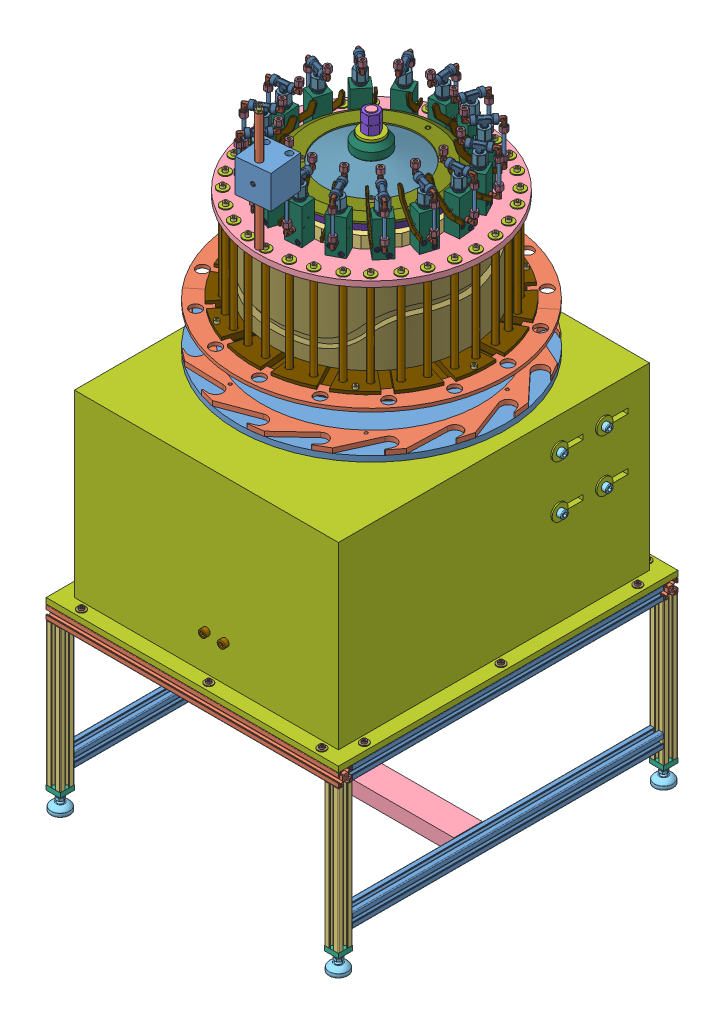
SolidWorks assembly Assieme_FINALE, configuration Default. Lengths in mm. (continued)
Components (placement in the parent): (continued)
- assieme parte rotante-2: assieme parte rotante [Default] at (-79.201 623.9178 -645.7922) x (0 1 0) z (-0.73003 0 0.683415) size (749.63 778.63 778.63) (continued)
  - AssiemeValvola-16: AssiemeValvola [Default] at (515.3257 153.2338 311.5106) x (0 -0.793353 0.608761) z (0 0.608761 0.793353) size (90.26 138.63 38) (continued)
    - Raccordo a L-2: Raccordo a L [Default] at (30 0 0) x (0 1 0) z (0 0 -1) size (28.34 25.51 14.01)
      - 1809_06_10_01-1: 1809_06_10_01 [Default] at origin size (22.49 23 10)
      - 1809_06_10_02-1: 1809_06_10_02 [Default] at origin size (6.5 8.5 8.5)
      - 1809_06_10_03-1: 1809_06_10_03 [Default] at origin size (11.02 15.01 14.01)
    - TappoChiusura-1: TappoChiusura [Default] at (0 -32 0) x (0 -1 0) z (0 0 1) size (38.28 26.74 26.74)
    - CorpoValvola-1: CorpoValvola [Default] at (-15 -115.2824 0) size (30 75 34)
    - Raccordo a L-3: Raccordo a L [Default] at (-30 -88.2824 0) x (0 1 0) z (0 0 1) size (28.34 25.51 14.01)
      - 1809_06_10_01-1: 1809_06_10_01 [Default] at origin size (22.49 23 10)
      - 1809_06_10_02-1: 1809_06_10_02 [Default] at origin size (6.5 8.5 8.5)
      - 1809_06_10_03-1: 1809_06_10_03 [Default] at origin size (11.02 15.01 14.01)
    - Spina_3x38-1: Spina_3x38 [Default] at (0 -68.2824 -21) x (-1 0 0) z (0 0 1) size (3 3 38)
    - Spina_3x38-2: Spina_3x38 [Default] at (-10 -80.2824 -21) x (0.996193 0.087174 0) z (0 0 1) size (3 3 38)
    - M5 40mm-3: M5 40mm [ISO 4762 M5 x 40 - 40N] at (-14.6 -108.7824 9) size (45 8.5 8.5)
    - M5 40mm-2: M5 40mm [ISO 4762 M5 x 40 - 40N] at (-14.6 -96.7824 -9) size (45 8.5 8.5)
    - LevaValvola-1: LevaValvola [Default] at (-24.507 -86.571 -17) x (0.996193 0.087174 0) z (0 0 1) size (77.55 60.2 4)
    - Tubo-1: Tubo [Default] at (-30 -15.9665 0) x (1 0 0) z (0 -1 0) size (6 6 56.4)
  - Disco alimentazione guarnizione fi24.4-1: Disco alimentazione guarnizione fi24.4 [Default] at (198.0433 18.3637 415) x (0 0.065403 0.997859) z (-1 0 0) size (570 285 7.35)
  - Disco alimentazione guarnizione fi24.4-2: Disco alimentazione guarnizione fi24.4 [Default] at (198.0433 18.3637 415) x (0 -0.065403 -0.997859) z (-1 0 0) size (570 285 7.35)
  - m6 12mm-1: m6 12mm [ISO 4762 M6 x 12 - 12N] at (210.0433 200.6849 574.8914) x (-1 0 0) z (0 0.793353 -0.608761) size (18 10 10)
  - m6 12mm-7: m6 12mm [ISO 4762 M6 x 12 - 12N] at (210.0433 260.3445 399.1397) x (-1 0 0) z (0 0.793353 -0.608761) size (18 10 10)
  - m6 12mm-8: m6 12mm [ISO 4762 M6 x 12 - 12N] at (210.0433 96.3128 185.3694) x (-1 0 0) z (0 0.793353 -0.608761) size (18 10 10)
  - m6 12mm-9: m6 12mm [ISO 4762 M6 x 12 - 12N] at (210.0433 -59.5854 644.6306) x (-1 0 0) z (0 -0.793353 -0.608761) size (18 10 10)
  - m6 12mm-10: m6 12mm [ISO 4762 M6 x 12 - 12N] at (210.0433 -223.6171 430.8603) x (-1 0 0) z (0 -0.793353 -0.608761) size (18 10 10)
  - m6 12mm-11: m6 12mm [ISO 4762 M6 x 12 - 12N] at (210.0433 -163.9575 255.1086) x (-1 0 0) z (0 0.793353 -0.608761) size (18 10 10)
- assieme parte fissa-1: assieme parte fissa [Default] at (-1179.2365 708.9757 -309.8267) x (0 -1 0) z (1 0 0) size (784.52 415.1 415.07)
  - AlberoPortaCamme-1: AlberoPortaCamme [Default] at (-462.1354 65.7544 784.523) size (784.52 50 50)
  - linguetta_uni_6604_a_14x9x150-1: linguetta_uni_6604_a_14x9x150 [Default] at (-282.1354 65.7544 802.023) x (1 0 0) z (0 -1 0) size (150 9 14)
  - linguetta_uni_6604_a_8x7x50-1: linguetta_uni_6604_a_8x7x50 [Default] at (-397.1354 65.7544 802.523) x (1 0 0) z (0 1 0) size (50 7 8)
  - linguetta_uni_6604_a_8x7x50-2: linguetta_uni_6604_a_8x7x50 [Default] at (-397.1354 65.7544 766.523) x (1 0 0) z (0 -1 0) size (50 7 8)
  - rondella 20d 50D 5mm-1: rondella 20d 50D 5mm [Default] at (-417.3639 65.7544 784.523) x (0 0 1) z (-1 0 0) size (50 50 5)
  - dado M20-3: dado M20 [ISO - 4034 - M20 - N] at (-441.3639 65.7544 784.523) x (0 -1 0) z (1 0 0) size (30 34.64 19)
  - dado M20-2: dado M20 [ISO - 4034 - M20 - N] at (-422.3639 65.7544 784.523) x (0 -1 0) z (1 0 0) size (30 34.64 19)
  - seger 47-11: seger 47 [B27.7M - 3AM1-50] at (292.1646 65.7544 784.523) x (0 0 -1) z (1 0 0) size (54.93 58.5 1.6)
  - seger 47-12: seger 47 [B27.7M - 3AM1-50] at (272.8646 65.7544 784.523) x (0 0 1) z (-1 0 0) size (54.93 58.5 1.6)
  - seger 47-13: seger 47 [B27.7M - 3AM1-50] at (-120.5354 65.7544 784.523) x (0 0 -1) z (1 0 0) size (54.93 58.5 1.6)
  - seger 47-14: seger 47 [B27.7M - 3AM1-50] at (-104.4354 65.7544 784.523) x (0 0 1) z (-1 0 0) size (54.93 58.5 1.6)
  - seger 45mm-2: seger 45mm [seger 45mm] at (-289.9354 65.7544 784.523) x (0 1 0) z (-1 0 0) size (52.13 56.09 2.8)
  - seger 40mm-3: seger 40mm [B27.8M - 3DM1-40] at (-342.1354 65.7544 784.523) x (0 -1 0) z (1 0 0) size (46.31 50.39 2.8)
  - camma-1: camma [Default] at (-135.1932 65.7544 784.523) x (0 1 0) z (0 0 1) size (415.1 160.05 415.07)
  - SKF - 6010 - 18,DE,NC,18_68-1: SKF - 6010 - 18,DE,NC,18_68 [SKF - 6010 - 18,DE,NC,18_68] at (282.5646 65.7544 784.523) size (16 80 80)
  - SKF - 6010 - 18,DE,NC,18_68-2: SKF - 6010 - 18,DE,NC,18_68 [SKF - 6010 - 18,DE,NC,18_68] at (-112.5354 65.7544 784.523) size (16 80 80)
  - assieme molla e distributore-2: assieme molla e distributore [Default] at (-388.2308 60.5069 994.523) x (0 -1 0) z (0 0 -1) size (295 75.23 295)
    - molla a tazza-1: molla a tazza [Default] at (-5.2475 5.9046 210) size (200 27.84 200)
    - flangia copertura molla-1: flangia copertura molla [Default] at (-5.2475 11.1331 210) size (70 28.5 70)
    - distributore_fisso-1: distributore_fisso [Default] at (-5.2475 -46.0954 210) x (1 0 0) z (0 1 0) size (295 295 47)
    - delring_distributore_fisso-1: delring_distributore_fisso [Default] at (-5.2475 -46.0954 210) x (0 0 1) z (0 1 0) size (295 295 12)
    - O-ring 12.5x1.8-A-ISO 3601-1-2: O-ring 12.5x1.8-A-ISO 3601-1 [O-ring 12.5x1.8-A-ISO 3601-1] at (-125.2475 -33.1954 210) x (0.868916 0 -0.49496) z (0 1 0) size (16.1 16.1 1.8)
    - M6 16mm-6: M6 16mm [ISO 4762 M6 x 16 - 16N] at (-79.4937 -15.0954 135.7538) x (0 -1 0) z (0 0 1) size (22 10 10)
    - M6 16mm-7: M6 16mm [ISO 4762 M6 x 16 - 16N] at (-79.4937 -15.0954 284.2462) x (0 -1 0) z (1 0 0) size (22 10 10)
    - M6 16mm-8: M6 16mm [ISO 4762 M6 x 16 - 16N] at (68.9987 -15.0954 284.2462) x (0 -1 0) z (0 0 -1) size (22 10 10)
    - M6 16mm-9: M6 16mm [ISO 4762 M6 x 16 - 16N] at (68.9987 -15.0954 135.7538) x (0 -1 0) z (-1 0 0) size (22 10 10)
- assieme_carrello_movimento-1: assieme_carrello_movimento [Default] at (-359.1807 1115.6198 -132.5608) x (0.995209 0 -0.097775) z (0 1 0) size (70 82 262.71)
  - carello movimento alternativo-1: carello movimento alternativo [Default] at (-11.6011 0.1165 35) size (70 70 70)
  - tubo_carello-1: tubo_carello [Default] at (-11.6011 -19.6699 70) x (0 -1 0) z (0 0 1) size (14 14 250)
  - raccordo dritto-1: raccordo dritto [Default] at (-11.6011 -19.6699 191.1) x (-1 0 0) z (0 1 0) size (14 16.61 13)
  - grano M8 12mm p-1: grano M8 12mm p [ISO 4026 - M8 x 12-N] at (-11.6011 -34.6699 70) x (0 1 0) z (0.714486 0 -0.69965) size (12 8 8)
  - SKF_KR_19_PPA-1: SKF_KR_19_PPA [Default] at (-11.6011 47.3301 70) x (0 -1 0) z (-0.951057 0 0.309017) size (32 19 19)
Mates (geometry in assembly coordinates):
- Parallelo2: parallel aligned: plane of SupportoBase_Totale-2 through (4.0127 -14.4529 -3.9361) normal (0 1 0)
- Perpendicolare1: perpendicular: plane of SupportoBase_Totale-2 through (4.0127 -14.4529 -3.9361) normal (0 1 0)
- Parallelo4: parallel aligned: plane of SupportoBase_Totale-2 through (4.0127 -14.4529 -3.9361) normal (0 0 1)
- Coincidente5: coincident anti-aligned: plane of SupportoBase_Totale-2/assieme_base-1/Supporto di Base per macchina-1 through (-154.7135 275.9611 -15.5811) normal (-1 0 0); plane of motoriduttore-1 through (-154.7135 275.9611 -1137.0941) normal (1 0 0)
- Tangente1: tangent anti-aligned: plane of SupportoBase_Totale-2/assieme_base-1/Supporto di Base per macchina-1 through (-93.2286 597.9611 -659.5811) normal (0 1 0); cylinder of motoriduttore-1 through (-154.7135 603.4611 -608.0941) axis (-1 0 0) radius 5.5
- Concentrico1: concentric anti-aligned: cylinder of motoriduttore-1 through (-267.2135 442.7547 -555.0941) axis (0 1 0) radius 15; cylinder of Assieme_Riduttore-1/AlberoRiduttore-1 through (-267.2135 379.4375 -555.0941) axis (0 -1 0) radius 12.5
- Coincidente9: coincident anti-aligned: plane of motoriduttore-1 through (-164.7135 602.1811 -1137.0941) normal (0 1 0); plane of Assieme_Riduttore-1/Rondella di fermo-2 through (-267.2135 602.1811 -555.0941) normal (0 -1 0)
- Coincidente12: coincident anti-aligned: plane of M10 50mm-1 through (-131.7135 606.5159 -520.4879) normal (-1 0 0); plane of plain washer xlarge grade c_iso-1 through (-131.7135 596.9697 -497.3823) normal (1 0 0)
- Concentrico4: concentric aligned: cylinder of M10 50mm-1 through (-89.9635 603.4611 -513.0941) axis (1 0 0) radius 5; cylinder of plain washer xlarge grade c_iso-1 through (-99.7885 603.4611 -513.0941) axis (1 0 0) radius 5.5
- Coincidente13: coincident anti-aligned: plane of M10 50mm-2 through (-131.7135 484.4611 -513.0941) normal (-1 0 0); plane of plain washer xlarge grade c_iso-2 through (-131.7135 475.4611 -513.0941) normal (1 0 0)
- Concentrico5: concentric aligned: cylinder of M10 50mm-2 through (-89.9635 492.4611 -513.0941) axis (1 0 0) radius 5; cylinder of plain washer xlarge grade c_iso-2 through (-99.7885 492.4611 -513.0941) axis (1 0 0) radius 5.5
- Coincidente14: coincident anti-aligned: plane of M10 50mm-5 through (-131.7135 595.4611 -608.0941) normal (-1 0 0); plane of plain washer xlarge grade c_iso-4 through (-131.7135 586.4611 -608.0941) normal (1 0 0)
- Concentrico6: concentric aligned: cylinder of M10 50mm-5 through (-89.9635 603.4611 -608.0941) axis (1 0 0) radius 5; cylinder of plain washer xlarge grade c_iso-4 through (-99.7885 603.4611 -608.0941) axis (1 0 0) radius 5.5
- Coincidente15: coincident anti-aligned: plane of M10 50mm-4 through (-131.7135 484.4611 -608.0941) normal (-1 0 0); plane of plain washer xlarge grade c_iso-3 through (-131.7135 475.4611 -608.0941) normal (1 0 0)
- Concentrico7: concentric aligned: cylinder of M10 50mm-4 through (-89.9635 492.4611 -608.0941) axis (1 0 0) radius 5; cylinder of plain washer xlarge grade c_iso-3 through (-99.7885 492.4611 -608.0941) axis (1 0 0) radius 5.5
- Concentrico8: concentric anti-aligned: cylinder of motoriduttore-1 through (-154.7135 603.4611 -608.0941) axis (-1 0 0) radius 5.5; cylinder of M10 50mm-5 through (-89.9635 603.4611 -608.0941) axis (1 0 0) radius 5
- Coincidente16: coincident anti-aligned: plane of SupportoBase_Totale-2/assieme_base-1/Supporto di Base per macchina-1 through (-134.7135 287.9611 -15.5811) normal (1 0 0); plane of plain washer xlarge grade c_iso-4 through (-134.7135 597.9611 -608.0941) normal (-1 0 0)
- Concentrico9: concentric anti-aligned: cylinder of motoriduttore-1 through (-154.7135 603.4611 -513.0941) axis (-1 0 0) radius 5.5; cylinder of M10 50mm-1 through (-89.9635 603.4611 -513.0941) axis (1 0 0) radius 5
- Coincidente17: coincident anti-aligned: plane of SupportoBase_Totale-2/assieme_base-1/Supporto di Base per macchina-1 through (-134.7135 287.9611 -15.5811) normal (1 0 0); plane of plain washer xlarge grade c_iso-1 through (-134.7135 601.3609 -508.0109) normal (-1 0 0)
- Coincidente18: coincident anti-aligned: plane of SupportoBase_Totale-2/assieme_base-1/Supporto di Base per macchina-1 through (-134.7135 287.9611 -15.5811) normal (1 0 0); plane of plain washer xlarge grade c_iso-3 through (-134.7135 486.9611 -608.0941) normal (-1 0 0)
- Concentrico10: concentric aligned: circle of motoriduttore-1; cylinder of M10 50mm-4 through (-89.9635 492.4611 -608.0941) axis (1 0 0) radius 5
- Coincidente19: coincident anti-aligned: plane of SupportoBase_Totale-2/assieme_base-1/Supporto di Base per macchina-1 through (-134.7135 287.9611 -15.5811) normal (1 0 0); plane of plain washer xlarge grade c_iso-2 through (-134.7135 486.9611 -513.0941) normal (-1 0 0)
- Concentrico11: concentric aligned: circle of motoriduttore-1; cylinder of M10 50mm-2 through (-89.9635 492.4611 -513.0941) axis (1 0 0) radius 5
- Concentrico12: concentric anti-aligned: cylinder of M10 50mm-4 through (-89.9635 492.4611 -608.0941) axis (1 0 0) radius 5; cylinder of hex nut style 2 gradeab_iso-7 through (-164.7135 492.4611 -608.0941) axis (-1 0 0) radius 4.25
- Coincidente20: coincident anti-aligned: plane of motoriduttore-1 through (-164.7135 275.9611 -1137.0941) normal (-1 0 0); plane of hex nut style 2 gradeab_iso-7 through (-164.7135 501.6987 -608.0941) normal (1 0 0)
- Concentrico13: concentric anti-aligned: cylinder of M10 50mm-5 through (-89.9635 603.4611 -608.0941) axis (1 0 0) radius 5; cylinder of hex nut style 2 gradeab_iso-5 through (-164.7135 603.4611 -608.0941) axis (-1 0 0) radius 4.25
- Coincidente21: coincident aligned: plane of motoriduttore-1 through (-164.7135 275.9611 -1137.0941) normal (-1 0 0); circle of hex nut style 2 gradeab_iso-1
- Concentrico14: concentric anti-aligned: cylinder of M10 50mm-1 through (-89.9635 603.4611 -513.0941) axis (1 0 0) radius 5; cylinder of hex nut style 2 gradeab_iso-8 through (-164.7135 603.4611 -513.0941) axis (-1 0 0) radius 4.25
- Coincidente22: coincident anti-aligned: plane of motoriduttore-1 through (-164.7135 275.9611 -1137.0941) normal (-1 0 0); plane of hex nut style 2 gradeab_iso-8 through (-164.7135 612.6987 -513.0941) normal (1 0 0)
- Concentrico15: concentric anti-aligned: cylinder of M10 50mm-2 through (-89.9635 492.4611 -513.0941) axis (1 0 0) radius 5; cylinder of hex nut style 2 gradeab_iso-6 through (-164.7135 492.4611 -513.0941) axis (-1 0 0) radius 4.25
- Coincidente23: coincident anti-aligned: plane of motoriduttore-1 through (-164.7135 275.9611 -1137.0941) normal (-1 0 0); plane of hex nut style 2 gradeab_iso-6 through (-164.7135 501.6987 -513.0941) normal (1 0 0)
- Concentrico164: concentric anti-aligned: cylinder of SupportoBase_Totale-2/assieme_base-1/Traversa di blocco albero-1 through (-394.7135 362.1119 -360.5811) axis (0 1 0) radius 5.25; cylinder of assieme parte fissa-1/AlberoPortaCamme-1 through (-394.7135 386.9611 -360.5811) axis (0 -1 0) radius 4.5
- Coincidente26: coincident anti-aligned: plane of SupportoBase_Totale-2/assieme_base-1/Traversa di blocco albero-1 through (-427.2135 386.9611 -53.5811) normal (0 1 0); plane of assieme parte fissa-1/AlberoPortaCamme-1 through (-394.7135 386.9611 -400.5811) normal (0 -1 0)
- Concentrico1651: concentric aligned: cylinder of SupportoBase_Totale-2/assieme_base-1/Traversa di blocco albero-1 through (-394.7135 362.1119 -360.5811) axis (0 1 0) radius 5.25; cylinder of rondella M8-1 through (-394.7135 374.9611 -360.5811) axis (0 1 0) radius 4.65
- Coincidente271: coincident anti-aligned: plane of SupportoBase_Totale-2/assieme_base-1/Traversa di blocco albero-1 through (-427.2135 376.9611 -53.5811) normal (0 -1 0); plane of rondella M8-1 through (-394.7135 376.9611 -360.5811) normal (0 1 0)
- Concentrico1661: concentric aligned: cylinder of SupportoBase_Totale-2/assieme_base-1/Traversa di blocco albero-1 through (-394.7135 362.1119 -390.5811) axis (0 1 0) radius 5.25; cylinder of rondella M8-2 through (-394.7135 374.9611 -390.5811) axis (0 1 0) radius 4.65
- Coincidente281: coincident anti-aligned: plane of SupportoBase_Totale-2/assieme_base-1/Traversa di blocco albero-1 through (-427.2135 376.9611 -53.5811) normal (0 -1 0); plane of rondella M8-2 through (-394.7135 376.9611 -390.5811) normal (0 1 0)
- Coincidente29: coincident aligned: plane of rondella M8-1 through (-394.7135 376.9611 -360.5811) normal (-1 0 0); plane of rondella M8-2 through (-394.7135 376.9611 -390.5811) normal (-1 0 0)
- Concentrico16621: concentric anti-aligned: cylinder of SupportoBase_Totale-2/assieme_base-1/Traversa di blocco albero-1 through (-394.7135 362.1119 -390.5811) axis (0 1 0) radius 5.25; cylinder of M8 25 mm-1 through (-394.7135 337.2111 -390.5811) axis (0 -1 0) radius 6.5
- Coincidente2821: coincident anti-aligned: plane of SupportoBase_Totale-2/assieme_base-1/Traversa di blocco albero-1 through (-427.2135 376.9611 -53.5811) normal (0 -1 0); plane of M8 25 mm-1 through (-400.3427 376.9611 -387.3311) normal (0 1 0)
- Concentrico16631: concentric anti-aligned: cylinder of rondella M8-1 through (-394.7135 374.9611 -360.5811) axis (0 1 0) radius 4.65; cylinder of M8 25 mm-2 through (-394.7135 335.2111 -360.5811) axis (0 -1 0) radius 6.5
- Coincidente284: coincident anti-aligned: plane of rondella M8-1 through (-394.7135 374.9611 -360.5811) normal (0 -1 0); plane of M8 25 mm-2 through (-389.0844 374.9611 -363.8311) normal (0 1 0)
- Coincidente285: coincident aligned: plane of M8 25 mm-1 through (-391.666 372.9611 -388.8216) normal (-1 0 0); plane of M8 25 mm-2 through (-391.666 370.9611 -362.3406) normal (-1 0 0)
- Concentrico16632: concentric aligned: cylinder of assieme parte rotante-1/asta scorrimento carello-15 through (-613.1413 1023.9611 -329.7302) axis (0 -1 0) radius 6; cylinder of assieme_carrello_movimento-1/carello movimento alternativo-1 through (-350.1176 1220.6198 -156.8936) axis (0 -1 0) radius 7
- Concentrico16635: concentric anti-aligned: cylinder of assieme parte rotante-1/asta scorrimento carello-30 through (-617.9018 798.9611 -375.4832) axis (0 1 0) radius 6; cylinder of assieme_carrello_movimento-1/carello movimento alternativo-1 through (-395.8972 1220.6198 -152.396) axis (0 -1 0) radius 7
- Concentrico16636: concentric aligned: cylinder of assieme parte rotante-1/asta scorrimento carello-16 through (-614.0609 1023.9611 -416.8091) axis (0 -1 0) radius 6; cylinder of assieme_carrello_movimento-2/carello movimento alternativo-1 through (-459.9272 910.3623 -161.953) axis (-0.033609 -0.99933 -0.014476) radius 7
- Concentrico16637: concentric anti-aligned: cylinder of assieme parte rotante-1/asta scorrimento carello-31 through (-600.95 798.9611 -460.9011) axis (0 1 0) radius 6; cylinder of assieme_carrello_movimento-2/carello movimento alternativo-1 through (-502.1467 912.0456 -180.1375) axis (-0.033609 -0.99933 -0.014476) radius 7
- Tangente3: tangent: face of ?; circle of ?
- Concentrico16638: concentric aligned: cylinder of assieme_carrello_movimento-3/carello movimento alternativo-1 through (-526.5316 917.3008 -192.7545) axis (-0.280699 -0.91554 -0.288088) radius 7; cylinder of assieme parte rotante-1/asta scorrimento carello-17 through (-581.5867 1023.9611 -497.6114) axis (0 -1 0) radius 6
- Concentrico16640: concentric anti-aligned: cylinder of assieme parte rotante-1/asta scorrimento carello-32 through (-552.6006 798.9611 -533.3298) axis (0 1 0) radius 6; cylinder of assieme_carrello_movimento-3/carello movimento alternativo-1 through (-555.9218 935.8032 -222.9186) axis (-0.280699 -0.91554 -0.288088) radius 7
- Concentrico16641: concentric aligned: cylinder of assieme parte rotante-1/asta scorrimento carello-1 through (-520.6629 1023.9611 -559.8357) axis (0 -1 0) radius 6; cylinder of assieme_carrello_movimento-4/carello movimento alternativo-1 through (-581.0889 958.1223 -248.6474) axis (-0.171686 -0.907744 -0.382787) radius 7
- Concentrico16642: concentric anti-aligned: cylinder of assieme parte rotante-1/asta scorrimento carello-2 through (-480.2144 798.9611 -581.7427) axis (0 1 0) radius 6; cylinder of assieme_carrello_movimento-4/carello movimento alternativo-1 through (-598.1769 977.4205 -286.747) axis (-0.171686 -0.907744 -0.382787) radius 7
- Tangente5: tangent: plane of assieme parte fissa-1/camma-1 through (-382.97 980.6111 -351.2489) normal (0 -1 0); circle of assieme_carrello_movimento-4/SKF_KR_19_PPA-1
- Tangente6: tangent: plane of assieme parte fissa-1/camma-1 through (-382.97 980.6111 -351.2489) normal (0 -1 0); circle of assieme_carrello_movimento-3/SKF_KR_19_PPA-1
- Concentrico16643: concentric anti-aligned: cylinder of assieme parte rotante-1/asta scorrimento carello-18 through (-394.8114 798.9611 -598.7693) axis (0 1 0) radius 6; cylinder of assieme_carrello_movimento-5/carello movimento alternativo-1 through (-617.2897 991.4532 -391.0444) axis (-0.00051 -0.999861 -0.016676) radius 7
- Concentrico16644: concentric aligned: cylinder of assieme parte rotante-1/asta scorrimento carello-3 through (-440.5644 1023.9611 -594.0089) axis (0 -1 0) radius 6; cylinder of assieme_carrello_movimento-5/carello movimento alternativo-1 through (-615.8849 990.6857 -345.0723) axis (-0.00051 -0.999861 -0.016676) radius 7
- Tangente7: tangent: plane of assieme parte fissa-1/camma-1 through (-382.97 980.6111 -351.2489) normal (0 -1 0); circle of assieme_carrello_movimento-5/SKF_KR_19_PPA-1
- Concentrico16645: concentric aligned: cylinder of assieme parte rotante-1/asta scorrimento carello-4 through (-353.4855 1023.9611 -594.9284) axis (0 -1 0) radius 6; cylinder of assieme_carrello_movimento-8/carello movimento alternativo-1 through (-499.9334 991.1064 -572.4113) axis (0.000166 -1 -0.000068) radius 7
- Concentrico16646: concentric aligned: cylinder of assieme parte rotante-1/asta scorrimento carello-5 through (-272.6832 1023.9611 -562.4543) axis (0 -1 0) radius 6; cylinder of assieme_carrello_movimento-7/carello movimento alternativo-1 through (-568.9143 991.108 -515.1065) axis (0.00008 -1 -0.000081) radius 7
- Concentrico16647: concentric anti-aligned: cylinder of assieme parte rotante-1/asta scorrimento carello-19 through (-309.3935 798.9611 -581.8176) axis (0 1 0) radius 6; cylinder of assieme_carrello_movimento-8/carello movimento alternativo-1 through (-457.3466 991.1146 -589.8) axis (0.000166 -1 -0.000068) radius 7
- Concentrico16648: concentric aligned: cylinder of assieme parte fissa-1/AlberoPortaCamme-1 through (-394.7135 1275.1556 -375.5811) axis (0 1 0) radius 25; cylinder of assieme parte rotante-2/albero rotazione piatti-1 through (-394.7135 684.3308 -375.5811) axis (0 1 0) radius 35
- Coincidente2822: coincident anti-aligned: plane of SupportoBase_Totale-2/assieme_base-1/canotto di supporto-1 through (-394.7135 673.9611 -375.5811) normal (0 1 0); plane of assieme parte rotante-2/SKF - 6020 - 20,DE,NC,20_68-2 through (-377.4453 673.9611 -320.7353) normal (0 -1 0)
- Concentrico16650: concentric aligned: cylinder of SupportoBase_Totale-2/assieme_base-1/canotto di supporto-1 through (-394.7135 587.1745 -375.5811) axis (0 1 0) radius 67.5; cylinder of assieme parte fissa-1/AlberoPortaCamme-1 through (-394.7135 1275.1556 -375.5811) axis (0 1 0) radius 25
- Concentrico16651: concentric anti-aligned: cylinder of assieme parte rotante-2/asta scorrimento carello-23 through (-395.8972 798.9611 -152.396) axis (0 1 0) radius 6; cylinder of assieme_carrello_movimento-1/carello movimento alternativo-1 through (-395.8972 1220.6198 -152.396) axis (0 -1 0) radius 7
- Concentrico16652: concentric aligned: cylinder of assieme parte rotante-2/asta scorrimento carello-8 through (-350.1176 1023.9611 -156.8936) axis (0 -1 0) radius 6; cylinder of assieme_carrello_movimento-1/carello movimento alternativo-1 through (-350.1176 1220.6198 -156.8936) axis (0 -1 0) radius 7
